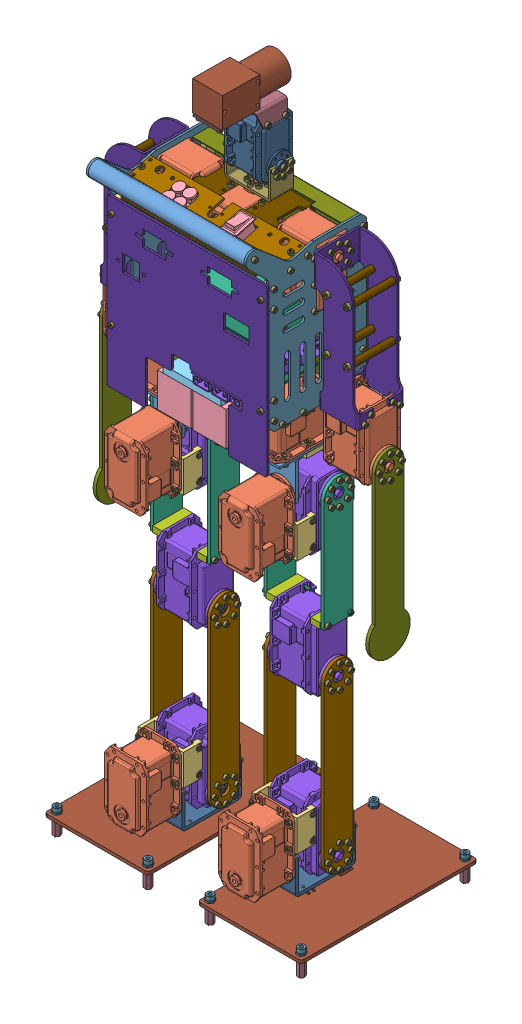
SolidWorks assembly 机器人, configuration 默认. Lengths in mm. (continued)
Mates (geometry in assembly coordinates): (continued)
- 重合73: coincident: plane of 右腿-1/机器人-髋关节连接件-1 through (1083.3402 413.4793 60.9843) normal (0 -1 0); plane of ? through (1083.3402 413.4793 71.9843) normal (0 1 0)
- 同心68: concentric: cylinder of 右腿-1/机器人-髋关节连接件-1 through (1075.562 416.4793 68.7625) axis (0 -1 0) radius 1.35; cylinder of ? through (1075.562 419.4793 68.7625) axis (0 -1 0) radius 1.25
- 重合74: coincident: plane of 右腿-1/机器人-髋关节连接件-1 through (1083.3402 413.4793 60.9843) normal (0 -1 0); plane of ? through (1075.562 413.4793 68.7625) normal (0 1 0)
- 同心69: concentric: cylinder of assembly; cylinder of assembly; cylinder of 手臂-2/机器人-上臂骨-1 through (1109.9402 578.8793 60.9843) axis (1 0 0) radius 5.5; cylinder of 躯干-1/MX64-4 through (1109.9402 578.8793 60.9843) axis (-1 0 0) radius 14
- 重合75: coincident: plane of assembly; plane of assembly; plane of 手臂-2/机器人-上臂骨-1 through (1109.9402 564.8793 90.9843) normal (-1 0 0); plane of 躯干-1/MX64-4 through (1109.9402 593.4393 46.4104) normal (1 0 0)
- 同心70: concentric: cylinder of assembly; cylinder of assembly; cylinder of 手臂-1/机器人-上臂骨-1 through (946.9402 578.8793 60.9843) axis (-1 0 0) radius 5.5; cylinder of 躯干-1/MX64-3 through (946.9402 578.8793 60.9843) axis (1 0 0) radius 14
- 重合76: coincident: plane of assembly; plane of assembly; plane of 手臂-1/机器人-上臂骨-1 through (946.9402 564.8793 30.9843) normal (1 0 0); plane of 躯干-1/MX64-3 through (946.9402 593.4393 75.5582) normal (-1 0 0)
- 平行1: parallel: plane of assembly; plane of assembly; plane of 手臂-2/机器人-上臂骨-1 through (1060.3129 564.8793 38.6116) normal (0 0 -1); plane of 躯干-1/机器人-前盖-2 through (1028.4402 526.9793 26.3843) normal (0 0 -1)
- 平行2: parallel: plane of assembly; plane of assembly; plane of 手臂-1/机器人-上臂骨-1 through (936.5675 564.8793 38.6116) normal (0 0 -1); plane of 躯干-1/机器人-前盖-2 through (1028.4402 526.9793 26.3843) normal (0 0 -1)
- 同心71: concentric: cylinder of 右腿-1/机器人-髋关节连接件-1 through (1083.3402 416.4793 60.9843) axis (0 -1 0) radius 6; cylinder of 躯干-1/MX64-1 through (1083.3402 414.6793 60.9843) axis (0 1 0) radius 5
- 同心72: concentric: cylinder of assembly; cylinder of assembly; cylinder of 左腿-1/机器人-髋关节连接件-1 through (973.5402 416.4793 60.9843) axis (0 -1 0) radius 6; cylinder of 躯干-1/MX64-2 through (973.5402 414.6793 60.9843) axis (0 1 0) radius 5
- 重合81: coincident: plane of assembly; plane of assembly; plane of 左腿-1/机器人-髋关节连接件-1 through (973.5402 416.4793 60.9843) normal (0 1 0); plane of 躯干-1/MX64-2 through (958.9663 416.4793 46.4243) normal (0 -1 0)
- 平行4: parallel: plane of assembly; plane of assembly; plane of 左腿-1/机器人-髋关节连接件-1 through (973.5402 443.7394 29.7643) normal (0 0 -1); plane of 躯干-1/机器人-前盖-2 through (1028.4402 526.9793 26.3843) normal (0 0 -1)
- 重合83: coincident: plane of 右腿-1/机器人-髋关节连接件-1 through (1083.3402 416.4793 60.9843) normal (0 1 0); plane of 躯干-1/MX64-1 through (1068.7663 416.4793 46.4243) normal (0 -1 0)
- 平行5: parallel: plane of 右腿-1/机器人-髋关节连接件-1 through (1083.3402 443.7394 29.7643) normal (0 0 -1); plane of 躯干-1/机器人-前盖-2 through (1028.4402 526.9793 26.3843) normal (0 0 -1)
- 同心74: concentric: cylinder of 右腿-1/机器人-髋关节连接件-1 through (1091.1184 416.4793 53.2061) axis (0 -1 0) radius 1.35; cylinder of ? through (1091.1184 419.4793 53.2061) axis (0 -1 0) radius 1.25
- 重合86: coincident: plane of 右腿-1/机器人-髋关节连接件-1 through (1083.3402 413.4793 60.9843) normal (0 -1 0); plane of ? through (1091.1184 413.4793 53.2061) normal (0 1 0)
- 同心75: concentric: cylinder of 右腿-1/机器人-髋关节连接件-1 through (1094.3402 416.4793 60.9843) axis (0 -1 0) radius 1.35; cylinder of ? through (1094.3402 419.4793 60.9843) axis (0 -1 0) radius 1.25
- 重合87: coincident: plane of 右腿-1/机器人-髋关节连接件-1 through (1083.3402 413.4793 60.9843) normal (0 -1 0); plane of ? through (1094.3402 413.4793 60.9843) normal (0 1 0)
- 同心76: concentric: cylinder of 右腿-1/机器人-髋关节连接件-1 through (1091.1184 416.4793 68.7625) axis (0 -1 0) radius 1.35; cylinder of ? through (1091.1184 419.4793 68.7625) axis (0 -1 0) radius 1.25
- 重合88: coincident: plane of 右腿-1/机器人-髋关节连接件-1 through (1083.3402 413.4793 60.9843) normal (0 -1 0); plane of ? through (1091.1184 413.4793 68.7625) normal (0 1 0)
- 同心77: concentric: cylinder of 右腿-1/机器人-髋关节连接件-1 through (1083.3402 416.4793 71.9843) axis (0 -1 0) radius 1.35; cylinder of ? through (1083.3402 419.4793 71.9843) axis (0 -1 0) radius 1.25
- 重合89: coincident: plane of 右腿-1/机器人-髋关节连接件-1 through (1083.3402 413.4793 60.9843) normal (0 -1 0); plane of ? through (1083.3402 413.4793 71.9843) normal (0 1 0)
- 同心78: concentric: cylinder of 右腿-1/机器人-髋关节连接件-1 through (1075.562 416.4793 68.7625) axis (0 -1 0) radius 1.35; cylinder of ? through (1075.562 419.4793 68.7625) axis (0 -1 0) radius 1.25
- 重合90: coincident: plane of 右腿-1/机器人-髋关节连接件-1 through (1083.3402 413.4793 60.9843) normal (0 -1 0); plane of ? through (1075.562 413.4793 68.7625) normal (0 1 0)
- 同心79: concentric: cylinder of 右腿-1/机器人-髋关节连接件-1 through (1072.3402 416.4793 60.9843) axis (0 -1 0) radius 1.35; cylinder of ? through (1072.3402 419.4793 60.9843) axis (0 -1 0) radius 1.25
- 重合91: coincident: plane of 右腿-1/机器人-髋关节连接件-1 through (1083.3402 413.4793 60.9843) normal (0 -1 0); plane of ? through (1072.3402 413.4793 60.9843) normal (0 1 0)
- 同心80: concentric: cylinder of 右腿-1/机器人-髋关节连接件-1 through (1075.562 416.4793 53.2061) axis (0 -1 0) radius 1.35; cylinder of ? through (1075.562 419.4793 53.2061) axis (0 -1 0) radius 1.25
- 重合92: coincident: plane of 右腿-1/机器人-髋关节连接件-1 through (1083.3402 413.4793 60.9843) normal (0 -1 0); plane of ? through (1075.562 413.4793 53.2061) normal (0 1 0)
- 同心81: concentric: cylinder of 右腿-1/机器人-髋关节连接件-1 through (1083.3402 416.4793 49.9843) axis (0 -1 0) radius 1.35; cylinder of ? through (1083.3402 419.4793 49.9843) axis (0 -1 0) radius 1.25
- 重合93: coincident: plane of 右腿-1/机器人-髋关节连接件-1 through (1083.3402 413.4793 60.9843) normal (0 -1 0); plane of ? through (1083.3402 413.4793 49.9843) normal (0 1 0)
- 同心82: concentric: cylinder of 左腿-1/机器人-髋关节连接件-1 through (973.5402 416.4793 49.9843) axis (0 -1 0) radius 1.35; cylinder of ? through (973.5402 419.4793 49.9843) axis (0 -1 0) radius 1.25
- 重合94: coincident: plane of 左腿-1/机器人-髋关节连接件-1 through (973.5402 413.4793 60.9843) normal (0 -1 0); plane of ? through (973.5402 413.4793 49.9843) normal (0 1 0)
- 同心83: concentric: cylinder of 左腿-1/机器人-髋关节连接件-1 through (981.3184 416.4793 53.2061) axis (0 -1 0) radius 1.35; cylinder of ? through (981.3184 419.4793 53.2061) axis (0 -1 0) radius 1.25
- 重合95: coincident: plane of 左腿-1/机器人-髋关节连接件-1 through (973.5402 413.4793 60.9843) normal (0 -1 0); plane of ? through (981.3184 413.4793 53.2061) normal (0 1 0)
- 同心84: concentric: cylinder of 左腿-1/机器人-髋关节连接件-1 through (984.5402 416.4793 60.9843) axis (0 -1 0) radius 1.35; cylinder of ? through (984.5402 419.4793 60.9843) axis (0 -1 0) radius 1.25
- 重合96: coincident: plane of 左腿-1/机器人-髋关节连接件-1 through (973.5402 413.4793 60.9843) normal (0 -1 0); plane of ? through (984.5402 413.4793 60.9843) normal (0 1 0)
- 同心85: concentric: cylinder of 左腿-1/机器人-髋关节连接件-1 through (981.3184 416.4793 68.7625) axis (0 -1 0) radius 1.35; cylinder of ? through (981.3184 419.4793 68.7625) axis (0 -1 0) radius 1.25
- 重合97: coincident: plane of 左腿-1/机器人-髋关节连接件-1 through (973.5402 413.4793 60.9843) normal (0 -1 0); plane of ? through (981.3184 413.4793 68.7625) normal (0 1 0)
- 同心86: concentric: cylinder of 左腿-1/机器人-髋关节连接件-1 through (973.5402 416.4793 71.9843) axis (0 -1 0) radius 1.35; cylinder of ? through (973.5402 419.4793 71.9843) axis (0 -1 0) radius 1.25
- 重合98: coincident: plane of 左腿-1/机器人-髋关节连接件-1 through (973.5402 413.4793 60.9843) normal (0 -1 0); plane of ? through (973.5402 413.4793 71.9843) normal (0 1 0)
- 同心87: concentric: cylinder of 左腿-1/机器人-髋关节连接件-1 through (965.762 416.4793 68.7625) axis (0 -1 0) radius 1.35; cylinder of ? through (965.762 419.4793 68.7625) axis (0 -1 0) radius 1.25
- 重合99: coincident: plane of 左腿-1/机器人-髋关节连接件-1 through (973.5402 413.4793 60.9843) normal (0 -1 0); plane of ? through (965.762 413.4793 68.7625) normal (0 1 0)
- 同心88: concentric: cylinder of 左腿-1/机器人-髋关节连接件-1 through (962.5402 416.4793 60.9843) axis (0 -1 0) radius 1.35; cylinder of ? through (962.5402 419.4793 60.9843) axis (0 -1 0) radius 1.25
- 重合100: coincident: plane of 左腿-1/机器人-髋关节连接件-1 through (973.5402 413.4793 60.9843) normal (0 -1 0); plane of ? through (962.5402 413.4793 60.9843) normal (0 1 0)
- 同心89: concentric: cylinder of 左腿-1/机器人-髋关节连接件-1 through (965.762 416.4793 53.2061) axis (0 -1 0) radius 1.35; cylinder of ? through (965.762 419.4793 53.2061) axis (0 -1 0) radius 1.25
- 重合101: coincident: plane of 左腿-1/机器人-髋关节连接件-1 through (973.5402 413.4793 60.9843) normal (0 -1 0); plane of ? through (965.762 413.4793 53.2061) normal (0 1 0)
- 同心90: concentric: cylinder of assembly; cylinder of assembly; cylinder of 手臂-2/机器人-上臂骨-1 through (1153.4856 467.8793 44.0843) axis (-1 0 0) radius 1.35; cylinder of hexagon socket head cap screws gb-81 through (1145.4856 467.8793 44.0843) axis (1 0 0) radius 1.25
- 重合102: coincident: plane of assembly; plane of assembly; plane of 手臂-2/机器人-上臂骨-1 through (1153.4856 564.8793 -51.8157) normal (1 0 0); plane of hexagon socket head cap screws gb-81 through (1153.4856 467.8793 44.0843) normal (-1 0 0)
- 同心91: concentric: cylinder of assembly; cylinder of assembly; cylinder of 手臂-2/机器人-上臂骨-1 through (1153.4856 473.1793 50.3843) axis (-1 0 0) radius 1.35; cylinder of hexagon socket head cap screws gb-82 through (1145.4856 473.1793 50.3843) axis (1 0 0) radius 1.25
- 重合103: coincident: plane of assembly; plane of assembly; plane of 手臂-2/机器人-上臂骨-1 through (1153.4856 564.8793 -51.8157) normal (1 0 0); plane of hexagon socket head cap screws gb-82 through (1153.4856 473.1793 50.3843) normal (-1 0 0)
- 同心92: concentric: cylinder of assembly; cylinder of assembly; cylinder of 手臂-2/机器人-上臂骨-1 through (1153.4856 473.1793 71.5843) axis (-1 0 0) radius 1.35; cylinder of hexagon socket head cap screws gb-83 through (1145.4856 473.1793 71.5843) axis (1 0 0) radius 1.25
- 重合104: coincident: plane of assembly; plane of assembly; plane of 手臂-2/机器人-上臂骨-1 through (1153.4856 564.8793 113.7843) normal (1 0 0); plane of hexagon socket head cap screws gb-83 through (1153.4856 473.1793 71.5843) normal (-1 0 0)
- 同心93: concentric: cylinder of assembly; cylinder of assembly; cylinder of 手臂-2/机器人-上臂骨-1 through (1153.4856 467.8793 77.8843) axis (-1 0 0) radius 1.35; cylinder of hexagon socket head cap screws gb-84 through (1145.4856 467.8793 77.8843) axis (1 0 0) radius 1.25
- 重合105: coincident: plane of assembly; plane of assembly; plane of 手臂-2/机器人-上臂骨-1 through (1153.4856 564.8793 113.7843) normal (1 0 0); plane of hexagon socket head cap screws gb-84 through (1153.4856 467.8793 77.8843) normal (-1 0 0)
- 同心94: concentric: cylinder of assembly; cylinder of assembly; cylinder of 手臂-2/机器人-上臂骨-1 through (1115.1402 467.8793 44.0843) axis (1 0 0) radius 1.35; cylinder of hexagon socket head cap screws gb-85 through (1123.1402 467.8793 44.0843) axis (-1 0 0) radius 1.25
- 重合106: coincident: plane of assembly; plane of assembly; plane of 手臂-2/机器人-上臂骨-1 through (1115.1402 564.8793 96.1843) normal (-1 0 0); plane of hexagon socket head cap screws gb-85 through (1115.1402 467.8793 44.0843) normal (1 0 0)
- 同心95: concentric: cylinder of assembly; cylinder of assembly; cylinder of 手臂-2/机器人-上臂骨-1 through (1115.1402 473.1793 50.3843) axis (1 0 0) radius 1.35; cylinder of hexagon socket head cap screws gb-86 through (1123.1402 473.1793 50.3843) axis (-1 0 0) radius 1.25
- 重合107: coincident: plane of assembly; plane of assembly; plane of 手臂-2/机器人-上臂骨-1 through (1115.1402 564.8793 96.1843) normal (-1 0 0); plane of hexagon socket head cap screws gb-86 through (1115.1402 473.1793 50.3843) normal (1 0 0)
- 同心96: concentric: cylinder of assembly; cylinder of assembly; cylinder of 手臂-2/机器人-上臂骨-1 through (1115.1402 473.1793 71.5843) axis (1 0 0) radius 1.35; cylinder of hexagon socket head cap screws gb-87 through (1123.1402 473.1793 71.5843) axis (-1 0 0) radius 1.25
- 重合108: coincident: plane of assembly; plane of assembly; plane of 手臂-2/机器人-上臂骨-1 through (1115.1402 564.8793 85.7843) normal (-1 0 0); plane of hexagon socket head cap screws gb-87 through (1115.1402 473.1793 71.5843) normal (1 0 0)
- 同心97: concentric: cylinder of assembly; cylinder of assembly; cylinder of 手臂-2/机器人-上臂骨-1 through (1115.1402 467.8793 77.8843) axis (1 0 0) radius 1.35; cylinder of hexagon socket head cap screws gb-88 through (1123.1402 467.8793 77.8843) axis (-1 0 0) radius 1.25
- 重合109: coincident: plane of assembly; plane of assembly; plane of 手臂-2/机器人-上臂骨-1 through (1115.1402 564.8793 85.7843) normal (-1 0 0); plane of hexagon socket head cap screws gb-88 through (1115.1402 467.8793 77.8843) normal (1 0 0)
- 同心98: concentric: cylinder of assembly; cylinder of assembly; cylinder of 手臂-1/机器人-上臂骨-1 through (903.3949 473.1793 71.5843) axis (1 0 0) radius 1.35; cylinder of hexagon socket head cap screws gb-89 through (911.3949 473.1793 71.5843) axis (-1 0 0) radius 1.25
- 重合110: coincident: plane of assembly; plane of assembly; plane of 手臂-1/机器人-上臂骨-1 through (903.3949 564.8793 173.7843) normal (-1 0 0); plane of hexagon socket head cap screws gb-89 through (903.3949 473.1793 71.5843) normal (1 0 0)
- 同心99: concentric: cylinder of assembly; cylinder of assembly; cylinder of 手臂-1/机器人-上臂骨-1 through (903.3949 467.8793 77.8843) axis (1 0 0) radius 1.35; cylinder of hexagon socket head cap screws gb-90 through (911.3949 467.8793 77.8843) axis (-1 0 0) radius 1.25
- 重合111: coincident: plane of assembly; plane of assembly; plane of 手臂-1/机器人-上臂骨-1 through (903.3949 564.8793 173.7843) normal (-1 0 0); plane of hexagon socket head cap screws gb-90 through (903.3949 467.8793 77.8843) normal (1 0 0)
- 同心100: concentric: cylinder of assembly; cylinder of assembly; cylinder of 手臂-1/机器人-上臂骨-1 through (903.3949 473.1793 50.3843) axis (1 0 0) radius 1.35; cylinder of hexagon socket head cap screws gb-91 through (911.3949 473.1793 50.3843) axis (-1 0 0) radius 1.25
- 重合112: coincident: plane of assembly; plane of assembly; plane of 手臂-1/机器人-上臂骨-1 through (903.3949 564.8793 8.1843) normal (-1 0 0); plane of hexagon socket head cap screws gb-91 through (903.3949 473.1793 50.3843) normal (1 0 0)
- 同心101: concentric: cylinder of assembly; cylinder of assembly; cylinder of 手臂-1/机器人-上臂骨-1 through (903.3949 467.8793 44.0843) axis (1 0 0) radius 1.35; cylinder of hexagon socket head cap screws gb-92 through (911.3949 467.8793 44.0843) axis (-1 0 0) radius 1.25
- 重合113: coincident: plane of assembly; plane of assembly; plane of 手臂-1/机器人-上臂骨-1 through (903.3949 564.8793 8.1843) normal (-1 0 0); plane of hexagon socket head cap screws gb-92 through (903.3949 467.8793 44.0843) normal (1 0 0)
- 同心102: concentric: cylinder of assembly; cylinder of assembly; cylinder of 手臂-1/机器人-上臂骨-1 through (941.7402 473.1793 71.5843) axis (-1 0 0) radius 1.35; cylinder of hexagon socket head cap screws gb-93 through (933.7402 473.1793 71.5843) axis (1 0 0) radius 1.25
- 重合114: coincident: plane of assembly; plane of assembly; plane of 手臂-1/机器人-上臂骨-1 through (941.7402 564.8793 25.7843) normal (1 0 0); plane of hexagon socket head cap screws gb-93 through (941.7402 473.1793 71.5843) normal (-1 0 0)
- 同心103: concentric: cylinder of assembly; cylinder of assembly; cylinder of 手臂-1/机器人-上臂骨-1 through (941.7402 467.8793 77.8843) axis (-1 0 0) radius 1.35; cylinder of hexagon socket head cap screws gb-94 through (933.7402 467.8793 77.8843) axis (1 0 0) radius 1.25
- 重合115: coincident: plane of assembly; plane of assembly; plane of 手臂-1/机器人-上臂骨-1 through (941.7402 564.8793 25.7843) normal (1 0 0); plane of hexagon socket head cap screws gb-94 through (941.7402 467.8793 77.8843) normal (-1 0 0)
- 同心104: concentric: cylinder of assembly; cylinder of assembly; cylinder of 手臂-1/机器人-上臂骨-1 through (941.7402 473.1793 50.3843) axis (-1 0 0) radius 1.35; cylinder of hexagon socket head cap screws gb-95 through (933.7402 473.1793 50.3843) axis (1 0 0) radius 1.25
- 重合116: coincident: plane of assembly; plane of assembly; plane of 手臂-1/机器人-上臂骨-1 through (941.7402 564.8793 36.1843) normal (1 0 0); plane of hexagon socket head cap screws gb-95 through (941.7402 473.1793 50.3843) normal (-1 0 0)
- 同心105: concentric: cylinder of assembly; cylinder of assembly; cylinder of 手臂-1/机器人-上臂骨-1 through (941.7402 467.8793 44.0843) axis (-1 0 0) radius 1.35; cylinder of hexagon socket head cap screws gb-96 through (933.7402 467.8793 44.0843) axis (1 0 0) radius 1.25
- 重合117: coincident: plane of assembly; plane of assembly; plane of 手臂-1/机器人-上臂骨-1 through (941.7402 564.8793 36.1843) normal (1 0 0); plane of hexagon socket head cap screws gb-96 through (941.7402 467.8793 44.0843) normal (-1 0 0)
- 同心106: concentric: cylinder of assembly; cylinder of assembly; cylinder of 手臂-2/机器人-上臂骨-1 through (1124.3129 564.8793 38.6116) axis (0 0 1) radius 1.6; cylinder of hexagon socket head cap screws gb-97 through (1124.3129 564.8793 44.6116) axis (0 0 -1) radius 1.5
- 重合118: coincident: plane of assembly; plane of assembly; plane of 手臂-2/机器人-上臂骨-1 through (1060.3129 564.8793 38.6116) normal (0 0 -1); plane of hexagon socket head cap screws gb-97 through (1124.3129 564.8793 38.6116) normal (0 0 1)
- 同心107: concentric: cylinder of assembly; cylinder of assembly; cylinder of 手臂-2/机器人-上臂骨-1 through (1144.3129 564.8793 38.6116) axis (0 0 1) radius 1.6; cylinder of hexagon socket head cap screws gb-98 through (1144.3129 564.8793 44.6116) axis (0 0 -1) radius 1.5
- 重合119: coincident: plane of assembly; plane of assembly; plane of 手臂-2/机器人-上臂骨-1 through (1060.3129 564.8793 38.6116) normal (0 0 -1); plane of hexagon socket head cap screws gb-98 through (1144.3129 564.8793 38.6116) normal (0 0 1)
- 同心108: concentric: cylinder of assembly; cylinder of assembly; cylinder of 手臂-2/机器人-上臂骨-1 through (1144.3129 514.8793 38.6116) axis (0 0 1) radius 1.6; cylinder of hexagon socket head cap screws gb-99 through (1144.3129 514.8793 44.6116) axis (0 0 -1) radius 1.5
- 重合120: coincident: plane of assembly; plane of assembly; plane of 手臂-2/机器人-上臂骨-1 through (1060.3129 564.8793 38.6116) normal (0 0 -1); plane of hexagon socket head cap screws gb-99 through (1144.3129 514.8793 38.6116) normal (0 0 1)
- 同心109: concentric: cylinder of assembly; cylinder of assembly; cylinder of 手臂-2/机器人-上臂骨-1 through (1124.3129 514.8793 38.6116) axis (0 0 1) radius 1.6; cylinder of hexagon socket head cap screws gb-100 through (1124.3129 514.8793 44.6116) axis (0 0 -1) radius 1.5
- 重合121: coincident: plane of assembly; plane of assembly; plane of 手臂-2/机器人-上臂骨-1 through (1060.3129 564.8793 38.6116) normal (0 0 -1); plane of hexagon socket head cap screws gb-100 through (1124.3129 514.8793 38.6116) normal (0 0 1)
- 同心110: concentric: cylinder of assembly; cylinder of assembly; cylinder of 手臂-2/机器人-上臂骨-1 through (1124.3129 564.8793 83.357) axis (0 0 -1) radius 1.6; cylinder of hexagon socket head cap screws gb-101 through (1124.3129 564.8793 77.357) axis (0 0 1) radius 1.5
- 重合122: coincident: plane of assembly; plane of assembly; plane of 手臂-2/机器人-上臂骨-1 through (1120.3129 564.8793 83.357) normal (0 0 1); plane of hexagon socket head cap screws gb-101 through (1124.3129 564.8793 83.357) normal (0 0 -1)
- 同心111: concentric: cylinder of assembly; cylinder of assembly; cylinder of 手臂-2/机器人-上臂骨-1 through (1144.3129 564.8793 83.357) axis (0 0 -1) radius 1.6; cylinder of hexagon socket head cap screws gb-102 through (1144.3129 564.8793 77.357) axis (0 0 1) radius 1.5
- 重合123: coincident: plane of assembly; plane of assembly; plane of 手臂-2/机器人-上臂骨-1 through (1120.3129 564.8793 83.357) normal (0 0 1); plane of hexagon socket head cap screws gb-102 through (1144.3129 564.8793 83.357) normal (0 0 -1)
- 同心112: concentric: cylinder of assembly; cylinder of assembly; cylinder of 手臂-2/机器人-上臂骨-1 through (1124.3129 514.8793 83.357) axis (0 0 -1) radius 1.6; cylinder of hexagon socket head cap screws gb-103 through (1124.3129 514.8793 77.357) axis (0 0 1) radius 1.5
- 重合124: coincident: plane of assembly; plane of assembly; plane of 手臂-2/机器人-上臂骨-1 through (1120.3129 564.8793 83.357) normal (0 0 1); plane of hexagon socket head cap screws gb-103 through (1124.3129 514.8793 83.357) normal (0 0 -1)
- 同心113: concentric: cylinder of assembly; cylinder of assembly; cylinder of 手臂-2/机器人-上臂骨-1 through (1144.3129 514.8793 83.357) axis (0 0 -1) radius 1.6; cylinder of hexagon socket head cap screws gb-104 through (1144.3129 514.8793 77.357) axis (0 0 1) radius 1.5
- 重合125: coincident: plane of assembly; plane of assembly; plane of 手臂-2/机器人-上臂骨-1 through (1120.3129 564.8793 83.357) normal (0 0 1); plane of hexagon socket head cap screws gb-104 through (1144.3129 514.8793 83.357) normal (0 0 -1)
- 同心114: concentric: cylinder of assembly; cylinder of assembly; cylinder of 手臂-1/机器人-上臂骨-1 through (912.5675 514.8793 83.357) axis (0 0 -1) radius 1.6; cylinder of hexagon socket head cap screws gb-105 through (912.5675 514.8793 77.357) axis (0 0 1) radius 1.5
- 重合126: coincident: plane of assembly; plane of assembly; plane of 手臂-1/机器人-上臂骨-1 through (996.5675 564.8793 83.357) normal (0 0 1); plane of hexagon socket head cap screws gb-105 through (912.5675 514.8793 83.357) normal (0 0 -1)
- 同心116: concentric: cylinder of assembly; cylinder of assembly; cylinder of 手臂-1/机器人-上臂骨-1 through (912.5675 564.8793 83.357) axis (0 0 -1) radius 1.6; cylinder of hexagon socket head cap screws gb-107 through (912.5675 564.8793 77.357) axis (0 0 1) radius 1.5
- 重合128: coincident: plane of assembly; plane of assembly; plane of 手臂-1/机器人-上臂骨-1 through (996.5675 564.8793 83.357) normal (0 0 1); plane of hexagon socket head cap screws gb-107 through (912.5675 564.8793 83.357) normal (0 0 -1)
- 同心117: concentric: cylinder of assembly; cylinder of assembly; cylinder of 手臂-1/机器人-上臂骨-1 through (932.5675 564.8793 83.357) axis (0 0 -1) radius 1.6; cylinder of hexagon socket head cap screws gb-108 through (932.5675 564.8793 77.357) axis (0 0 1) radius 1.5
- 重合129: coincident: plane of assembly; plane of assembly; plane of 手臂-1/机器人-上臂骨-1 through (996.5675 564.8793 83.357) normal (0 0 1); plane of hexagon socket head cap screws gb-108 through (932.5675 564.8793 83.357) normal (0 0 -1)
- 同心118: concentric: cylinder of assembly; cylinder of assembly; cylinder of 手臂-1/机器人-上臂骨-1 through (932.5675 514.8793 83.357) axis (0 0 -1) radius 1.6; cylinder of hexagon socket head cap screws gb-109 through (932.5675 514.8793 77.357) axis (0 0 1) radius 1.5
- 重合130: coincident: plane of assembly; plane of assembly; plane of 手臂-1/机器人-上臂骨-1 through (996.5675 564.8793 83.357) normal (0 0 1); plane of hexagon socket head cap screws gb-109 through (932.5675 514.8793 83.357) normal (0 0 -1)
- 同心119: concentric: cylinder of assembly; cylinder of assembly; cylinder of 手臂-1/机器人-上臂骨-1 through (932.5675 564.8793 38.6116) axis (0 0 1) radius 1.6; cylinder of hexagon socket head cap screws gb-110 through (932.5675 564.8793 44.6116) axis (0 0 -1) radius 1.5
- 重合131: coincident: plane of assembly; plane of assembly; plane of 手臂-1/机器人-上臂骨-1 through (936.5675 564.8793 38.6116) normal (0 0 -1); plane of hexagon socket head cap screws gb-110 through (932.5675 564.8793 38.6116) normal (0 0 1)
- 同心120: concentric: cylinder of assembly; cylinder of assembly; cylinder of 手臂-1/机器人-上臂骨-1 through (912.5675 564.8793 38.6116) axis (0 0 1) radius 1.6; cylinder of hexagon socket head cap screws gb-111 through (912.5675 564.8793 44.6116) axis (0 0 -1) radius 1.5
- 重合132: coincident: plane of assembly; plane of assembly; plane of 手臂-1/机器人-上臂骨-1 through (936.5675 564.8793 38.6116) normal (0 0 -1); plane of hexagon socket head cap screws gb-111 through (912.5675 564.8793 38.6116) normal (0 0 1)
- 同心121: concentric: cylinder of assembly; cylinder of assembly; cylinder of 手臂-1/机器人-上臂骨-1 through (932.5675 514.8793 38.6116) axis (0 0 1) radius 1.6; cylinder of hexagon socket head cap screws gb-112 through (932.5675 514.8793 44.6116) axis (0 0 -1) radius 1.5
- 重合133: coincident: plane of assembly; plane of assembly; plane of 手臂-1/机器人-上臂骨-1 through (936.5675 564.8793 38.6116) normal (0 0 -1); plane of hexagon socket head cap screws gb-112 through (932.5675 514.8793 38.6116) normal (0 0 1)
- 同心122: concentric: cylinder of assembly; cylinder of assembly; cylinder of 手臂-1/机器人-上臂骨-1 through (912.5675 514.8793 38.6116) axis (0 0 1) radius 1.6; cylinder of hexagon socket head cap screws gb-113 through (912.5675 514.8793 44.6116) axis (0 0 -1) radius 1.5
- 重合134: coincident: plane of assembly; plane of assembly; plane of 手臂-1/机器人-上臂骨-1 through (936.5675 564.8793 38.6116) normal (0 0 -1); plane of hexagon socket head cap screws gb-113 through (912.5675 514.8793 38.6116) normal (0 0 1)
